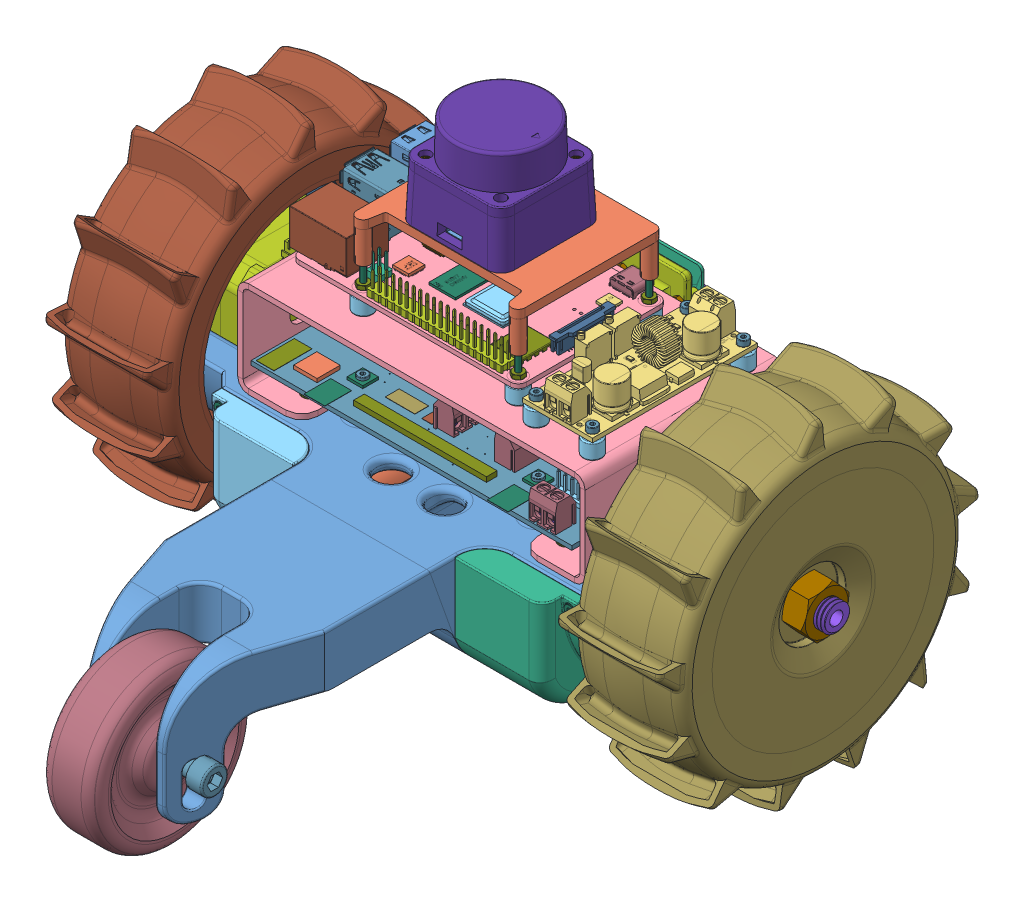
SolidWorks assembly RILey_assembly, configuration Default. Lengths in mm.
Overall size (244.39 192.08 262.82).
234 component instances, 82 part files, 220 mates.
Components (placement in the parent):
- MiddlepartV1-1: MiddlepartV1 [Middlepart_withoutTail] at origin size (201.11 74.9 106.82)
- MiddlepartV1-2: MiddlepartV1 [Tail] at origin size (60 50 93.64)
- 3_battery_pack-1: 3_battery_pack [Défaut] at (-114.6477 -13.5383 4.867) x (0.340955 0.94008 0) z (0.94008 -0.340955 0) size (33.05 64.4 54.62)
  - Li-ion Battery-1: Li-ion Battery [Défaut] at (13.1472 -31.5804 64) size (18 64.02 18)
  - link2-1: link2 [Défaut] at (30.5553 32.4196 84.2976) x (-0.340955 0 -0.94008) z (0 1 0) size (44 5 0.2)
  - Li-ion Battery-2: Li-ion Battery [Défaut] at (19.2844 -31.5804 80.9214) x (0.492149 0 0.870511) z (-0.870511 0 0.492149) size (18 64.02 18)
  - Li-ion Battery-3: Li-ion Battery [Défaut] at (25.4216 -31.5804 97.8429) x (0.922234 0 -0.386631) z (0.386631 0 0.922234) size (18 64.02 18)
  - link2-2: link2 [Défaut] at (25.7705 -31.5804 71.1051) x (0.340955 0 0.94008) z (0 -1 0) size (44 5 0.2)
- 3_battery_pack-2: 3_battery_pack [Défaut] at (-50.6477 -13.5383 4.867) x (0.340955 0.94008 0) z (0.94008 -0.340955 0) size (33.05 64.4 54.62)
  - Li-ion Battery-1: Li-ion Battery [Défaut] at (13.1472 -31.5804 64) size (18 64.02 18)
  - link2-1: link2 [Défaut] at (30.5553 32.4196 84.2976) x (-0.340955 0 -0.94008) z (0 1 0) size (44 5 0.2)
  - Li-ion Battery-2: Li-ion Battery [Défaut] at (19.2844 -31.5804 80.9214) x (0.492149 0 0.870511) z (-0.870511 0 0.492149) size (18 64.02 18)
  - Li-ion Battery-3: Li-ion Battery [Défaut] at (25.4216 -31.5804 97.8429) x (0.922234 0 -0.386631) z (0.386631 0 0.922234) size (18 64.02 18)
  - link2-2: link2 [Défaut] at (25.7705 -31.5804 71.1051) x (0.340955 0 0.94008) z (0 -1 0) size (44 5 0.2)
- BatteryCoverFront-1: BatteryCoverFront [Default] at (0 -39 -22) size (137.1 39.19 32.19)
- BatteryCoverBackLeft-1: BatteryCoverBackLeft [Default] at (-49.25 -40 30.5671) x (-1 0 0) z (0 0 -1) size (40.1 41.17 43.87)
- BatteryCoverBackRight-1: BatteryCoverBackRight [Default] at (49.25 -40 30.5671) x (-1 0 0) z (0 0 -1) size (40.1 41.17 43.86)
- Nema 17_Slim-1: Nema 17_Slim [Default] at (70.5 0 0) x (0 0 1) z (0 1 0) size (42 43 47.1)
- Nema 17_Slim-2: Nema 17_Slim [Default] at (-70.5 0 0) x (0 0 -1) z (0 1 0) size (42 43 47.1)
- LeftWheelAssembly-1: LeftWheelAssembly [Default] at (0.5 0 0) size (46.89 175.5 175.66)
  - HexBolt_modified-1: HexBolt_modified [Default] at (-101 0 0) x (0 0 1) z (-1 0 0) size (19.63 17 21.55)
  - hex nut style 1 gradeab_din-1: hex nut style 1 gradeab_din [Hexagon Nut ISO 4032 - M10 - D - S] at (-118.4 0 0) x (0 0 1) z (-1 0 0) size (16 18.48 8.4)
  - socket set screw cup point_din-1: socket set screw cup point_din [DIN 916 - M3 x 5-S] at (-104 7.5 0) x (0 -1 0) z (-0.467009 0 0.884252) size (5 3 3)
  - ReelyBuggyWheel_Left-2: ReelyBuggyWheel_Left [Default] at (-96.5 0 0) x (0 -0.851174 0.524883) z (-1 0 0) size (127.36 127.83 41.68)
- RightWheelAssembly-1: RightWheelAssembly [Default] at (68.7841 25.9686 -6.2213) x (-0.999996 0.002302 0.001897) z (-0.002983 -0.771739 -0.635933) size (47.18 164.08 164.48)
  - hex nut style 1 gradeab_din-2: hex nut style 1 gradeab_din [Hexagon Nut ISO 4032 - M10 - D - S] at (-40.7637 -21.3156 15.9632) x (0.002628 0.473226 -0.880937) z (0.999996 0 0.002983) size (16 18.48 8.4)
  - ReelyBuggyWheel_Right-1: ReelyBuggyWheel_Right [Default] at (-27.2638 -21.3156 16.0035) x (0.001045 0.936608 -0.350379) z (-0.999996 0 -0.002983) size (127.36 127.83 41.68)
  - socket set screw cup point_din-1: socket set screw cup point_din [DIN 916 - M3 x 5-S] at (-34.7467 -16.6097 10.2703) x (-0.002302 -0.635936 0.771739) z (-0.466048 0.683487 0.561824) size (5 3 3)
  - HexBolt_modified-1: HexBolt_modified [Default] at (-31.7638 -21.3156 15.9901) x (-0.001897 0.771742 0.635933) z (-0.999996 0 -0.002983) size (19.63 17 21.55)
- Backwheel-1: Backwheel [Default] at (0 -32.6496 136.5106) x (0 -0.126554 -0.99196) z (1 0 0) size (60 60 21)
- RILey_PCB-1: RILey_PCB [Default] at (48.6376 -44.5013 95.7539) x (-1 0 0) z (0 0 -1) size (120 19.05 71.04)
  - RILey_PCB.step-1: RILey_PCB.step [Default] at (-11.3624 54.5013 128.2539) x (1 0 0) z (0 1 0) size (120 71.04 11.3)
    - PCB Component.step-1: PCB Component.step [Default] at origin size (120 71.04 11.3)
      - Board.step-1: Board.step [Default] at origin size (120 70 1.57)
      - 0026604020.step-1: 0026604020.step [Default] at (95.25 66.04 1.57) size (7.77 10.01 0.1)
      - 0026604020.step-2: 0026604020.step [Default] at (26.67 66.04 1.57) size (7.77 10.01 0.1)
      - 2540-.step-1: 2540-.step [Default] at (61.27 63.5 1.57) size (49.68 3.96 1.83)
      - W237-102.step-1: W237-102.step [Default] at (11.481 64.491 1.57) x (-1 0 0) z (0 0 1) size (6.7 3.4 2.59)
      - W237-102.step-2: W237-102.step [Default] at (13.97 5.08 1.57) size (6.7 3.4 2.59)
      - W237-102.step-3: W237-102.step [Default] at (59.588 52.07 1.57) x (0 1 0) z (0 0 1) size (6.7 3.4 2.59)
      - W237-102.step-4: W237-102.step [Default] at (39.37 52.07 1.57) x (0 -1 0) z (0 0 1) size (6.7 3.4 2.59)
      - FE08-1_3D.step-1: FE08-1_3D.step [Default] at (26.67 31.75 1.57) x (0 1 0) z (0 0 1) size (20.82 2.5 11.3)
      - FE08-1_3D.step-2: FE08-1_3D.step [Default] at (12.7 31.75 1.57) x (0 1 0) z (0 0 1) size (20.82 2.5 11.3)
      - FE08-1_3D.step-3: FE08-1_3D.step [Default] at (93.98 27.94 1.57) x (0 -1 0) z (0 0 1) size (20.82 2.5 11.3)
      - FE08-1_3D.step-4: FE08-1_3D.step [Default] at (107.95 27.94 1.57) x (0 -1 0) z (0 0 1) size (20.82 2.5 11.3)
      - B4B-XH-A_LF__SN_.step-1: B4B-XH-A_LF__SN_.step [Default] at (5.08 27.94 1.57) x (0 1 0) z (0 0 1) size (12.9 6.25 0.1)
      - B4B-XH-A_LF__SN_.step-2: B4B-XH-A_LF__SN_.step [Default] at (115.57 31.75 1.57) x (0 -1 0) z (0 0 1) size (12.9 6.25 0.1)
      - 733980-62.step-1: 733980-62.step [Default] at (106.68 66.04 1.57) x (-1 0 0) z (0 0 1) size (8.75 8.65 1.36)
      - FE10-1_3D.step-1: FE10-1_3D.step [Default] at (66.04 15.259 1.57) x (0 -1 0) z (0 0 1) size (25.9 2.5 11.3)
      - FE04-1.step-1: FE04-1.step [Default] at (51.003 15.646 1.57) x (-1 0 0) z (0 0 1) size (10.16 2.5 11.3)
      - MA05-1_SMALLPAD.step-1: MA05-1_SMALLPAD.step [Default] at (13.97 55.88 1.57) x (-1 0 0) z (0 0 1) size (13.2 2.5 11)
      - 100uF.step-1: 100uF.step [Default] at (10.16 46.99 1.57) x (-1 0 0) z (0 0 1) size (7.55 7.55 0.1)
      - 100uF.step-2: 100uF.step [Default] at (97.79 43.18 1.57) size (7.55 7.55 0.1)
      - PTS18126V260.step-1: PTS18126V260.step [Default] at (62.23 40.64 0) x (0 1 0) z (0 0 -1) size (5.95 3.93 0.1)
      - MA04-1_SMALLPAD.step-1: MA04-1_SMALLPAD.step [Default] at (99.06 7.62 1.57) x (0 -1 0) z (0 0 1) size (10.66 2.5 11)
      - MA04-1_SMALLPAD.step-2: MA04-1_SMALLPAD.step [Default] at (104.14 7.62 1.57) x (0 -1 0) z (0 0 1) size (10.66 2.5 11)
      - MA04-1_SMALLPAD.step-3: MA04-1_SMALLPAD.step [Default] at (110.49 7.62 1.57) x (0 -1 0) z (0 0 1) size (10.66 2.5 11)
      - MA04-1_SMALLPAD.step-4: MA04-1_SMALLPAD.step [Default] at (115.57 7.62 1.57) x (0 -1 0) z (0 0 1) size (10.66 2.5 11)
      - MA04-1_SMALLPAD.step-5: MA04-1_SMALLPAD.step [Default] at (42.012 6.401 1.57) x (-1 0 0) z (0 0 1) size (10.66 2.5 11)
      - 1uF.step-1: 1uF.step [Default] at (85.09 36.83 1.57) x (0 -1 0) z (0 0 1) size (4.14 1.6 1.07)
      - 47uF.step-1: 47uF.step [Default] at (80.01 38.1 1.57) x (0 -1 0) z (0 0 1) size (6.68 1.6 0.99)
      - SA5.0A-E3_54.step-1: SA5.0A-E3_54.step [Default] at (67.31 55.88 1.57) x (0 -1 0) z (0 0 1) size (21.18 3.8 0.1)
      - IRF9530NPBF.step-1: IRF9530NPBF.step [Default] at (74.93 53.34 1.57) size (11.04 5.19 0.1)
      - BCM857BS,115.step-1: BCM857BS,115.step [Default] at (78.74 48.26 0) x (1 0 0) z (0 0 -1) size (3.4 2.7 0.1)
      - 10k.step-1: 10k.step [Default] at (74.93 40.64 1.57) x (0 1 0) z (0 0 1) size (10.6 2.5 4.42)
      - 10k.step-2: 10k.step [Default] at (72.39 40.64 1.57) x (0 1 0) z (0 0 1) size (10.6 2.5 4.42)
      - 2,8.step-1: 2,8.step [Default] at (27.15 9.65 1.57) size (5.84 5.84 0.97)
      - 2,8.step-2: 2,8.step [Default] at (92.85 55.35 1.57) size (5.84 5.84 0.97)
      - 2,8.step-3: 2,8.step [Default] at (27.15 55.35 1.57) size (5.84 5.84 0.97)
      - 2,8.step-4: 2,8.step [Default] at (92.85 9.65 1.57) size (5.84 5.84 0.97)
      - 1101M2S3CQE2.step-1: 1101M2S3CQE2.step [Default] at (115.621 62.763 1.57) size (6.6 14.23 0.1)
  - DRV 8825 With Headers Assem-1: DRV 8825 With Headers Assem [Default] at (18.6208 50.4495 104.6201) x (0 0 -1) z (0 1 0) size (21 15 10.9)
    - PCB-1: PCB [Default] at (8.1162 10.2982 16.4218) size (21 15 1.8)
    - SMD Pot-1: SMD Pot [Default] at (-0.2134 7.4613 18.0218) x (0 -1 0) z (0 0 1) size (3 3 1.3)
    - 0603 Resistor-1: 0603 Resistor [Default] at (-1.0068 10.8561 18.0218) size (1.5 0.8 0.5)
    - 0603 Resistor-2: 0603 Resistor [Default] at (-1.0286 12.2306 18.0218) size (1.5 0.8 0.5)
    - 0805 Capacitor-1: 0805 Capacitor [Default] at (-0.8941 14.0417 18.0218) size (2 1.25 1.25)
    - 0402 Resistor-1: 0402 Resistor [Default] at (16.8896 6.6863 18.0218) x (0 -1 0) z (0 0 1) size (1 0.68 0.66)
    - 0402 Resistor-2: 0402 Resistor [Default] at (16.8896 10.308 18.0218) x (0 -1 0) z (0 0 1) size (1 0.68 0.66)
    - 0402 Resistor-3: 0402 Resistor [Default] at (16.8896 13.6408 18.0218) x (0 -1 0) z (0 0 1) size (1 0.68 0.66)
    - 0402 Resistor-4: 0402 Resistor [Default] at (6.8882 6.5987 18.0218) x (0 -1 0) z (0 0 1) size (1 0.68 0.66)
    - 0402 Resistor-5: 0402 Resistor [Default] at (5.9719 6.5987 18.0218) x (0 -1 0) z (0 0 1) size (1 0.68 0.66)
    - 0402 Resistor-6: 0402 Resistor [Default] at (5.456 14.3274 18.0218) size (1 0.68 0.66)
    - 0402 Resistor-7: 0402 Resistor [Default] at (5.456 13.4855 18.0218) size (1 0.68 0.66)
    - DRV8825 IC-1: DRV8825 IC [Default] at (11.7347 10.2312 18.0218) x (0 -1 0) z (0 0 1) size (9.6 6.2 1.2)
    - 8 pin Header-1: 8 pin Header [Default] at (8.1162 16.2982 13.9218) size (21 2.5 10.5)
    - 8 pin Header-2: 8 pin Header [Default] at (8.1162 4.2982 13.9218) size (21 2.5 10.5)
  - DRV 8825 With Headers Assem-2: DRV 8825 With Headers Assem [Default] at (79.3044 50.4495 92.1976) x (0 0 1) z (0 1 0) size (21 15 10.9)
    - PCB-1: PCB [Default] at (8.1162 10.2982 16.4218) size (21 15 1.8)
    - SMD Pot-1: SMD Pot [Default] at (-0.2134 7.4613 18.0218) x (0 -1 0) z (0 0 1) size (3 3 1.3)
    - 0603 Resistor-1: 0603 Resistor [Default] at (-1.0068 10.8561 18.0218) size (1.5 0.8 0.5)
    - 0603 Resistor-2: 0603 Resistor [Default] at (-1.0286 12.2306 18.0218) size (1.5 0.8 0.5)
    - 0805 Capacitor-1: 0805 Capacitor [Default] at (-0.8941 14.0417 18.0218) size (2 1.25 1.25)
    - 0402 Resistor-1: 0402 Resistor [Default] at (16.8896 6.6863 18.0218) x (0 -1 0) z (0 0 1) size (1 0.68 0.66)
    - 0402 Resistor-2: 0402 Resistor [Default] at (16.8896 10.308 18.0218) x (0 -1 0) z (0 0 1) size (1 0.68 0.66)
    - 0402 Resistor-3: 0402 Resistor [Default] at (16.8896 13.6408 18.0218) x (0 -1 0) z (0 0 1) size (1 0.68 0.66)
    - 0402 Resistor-4: 0402 Resistor [Default] at (6.8882 6.5987 18.0218) x (0 -1 0) z (0 0 1) size (1 0.68 0.66)
    - 0402 Resistor-5: 0402 Resistor [Default] at (5.9719 6.5987 18.0218) x (0 -1 0) z (0 0 1) size (1 0.68 0.66)
    - 0402 Resistor-6: 0402 Resistor [Default] at (5.456 14.3274 18.0218) size (1 0.68 0.66)
    - 0402 Resistor-7: 0402 Resistor [Default] at (5.456 13.4855 18.0218) size (1 0.68 0.66)
    - DRV8825 IC-1: DRV8825 IC [Default] at (11.7347 10.2312 18.0218) x (0 -1 0) z (0 0 1) size (9.6 6.2 1.2)
    - 8 pin Header-1: 8 pin Header [Default] at (8.1162 16.2982 13.9218) size (21 2.5 10.5)
    - 8 pin Header-2: 8 pin Header [Default] at (8.1162 4.2982 13.9218) size (21 2.5 10.5)
  - MPU9250.STEP-2: MPU9250.STEP [Default] at (87.1776 67.9346 116.1747) x (0 0 1) z (-1 0 0) size (26 3.91 16)
    - PCB.STEP-1: PCB.STEP [Default] at (-2.9998 1.0768 26) size (26 2.2 16)
    - C2.STEP-1: C2.STEP [Default] at (-2.4989 2.0768 21) x (0 0 -1) z (1 0 0) size (2 1.81 5.01)
    - MP92.STEP-1: MP92.STEP [Default] at (-2.9998 1.0968 25.5) x (0 0 -1) z (1 0 0) size (3.29 1.01 3.29)
    - C1_Predeterminado_Como mecanizada_.STEP-1: C1_Predeterminado_Como mecanizada_.STEP [Default] at (2.1384 1.0968 23.0905) x (0 0 1) z (-1 0 0) size (2.2 0.83 0.9)
    - C1_Predeterminado_Como mecanizada_.STEP-2: C1_Predeterminado_Como mecanizada_.STEP [Default] at (0.9102 1.0968 27.1044) x (0 0 1) z (-1 0 0) size (2.2 0.83 0.9)
    - C1_Predeterminado_Como mecanizada_.STEP-3: C1_Predeterminado_Como mecanizada_.STEP [Default] at (0.9102 1.0968 23.0905) x (0 0 1) z (-1 0 0) size (2.2 0.83 0.9)
    - C1_Predeterminado_Como mecanizada_.STEP-4: C1_Predeterminado_Como mecanizada_.STEP [Default] at (-8.3098 1.0968 23.0905) x (0 0 1) z (-1 0 0) size (2.2 0.83 0.9)
    - C1_Predeterminado_Como mecanizada_.STEP-5: C1_Predeterminado_Como mecanizada_.STEP [Default] at (-9.7098 1.0968 27.1044) x (0 0 1) z (-1 0 0) size (2.2 0.83 0.9)
    - R1.STEP-1: R1.STEP [Default] at (3.5484 1.1168 27.2144) x (0 0 -1) z (1 0 0) size (2.2 0.47 0.9)
    - R1.STEP-2: R1.STEP [Default] at (2.1484 1.1168 27.2144) x (0 0 -1) z (1 0 0) size (2.2 0.47 0.9)
    - R1.STEP-3: R1.STEP [Default] at (-6.8998 1.1168 23.2005) x (0 0 -1) z (1 0 0) size (2.2 0.47 0.9)
    - R1.STEP-4: R1.STEP [Default] at (-8.2998 1.1168 27.2144) x (0 0 -1) z (1 0 0) size (2.2 0.47 0.9)
    - R1.STEP-5: R1.STEP [Default] at (-6.8998 1.1168 27.2144) x (0 0 -1) z (1 0 0) size (2.2 0.47 0.9)
    - V1.STEP-1: V1.STEP [Default] at (-13.0785 1.5868 25.9) size (2.9 0.96 3.2)
  - PinHeader10row-1: PinHeader10row [Default] at (53.4076 66.9113 102.8349) x (0 0 -1) z (-1 0 0) size (25.4 11.54 2.54)
  - DG301-5.0-02-1: DG301-5.0-02 [Default] at (0.1076 56.0713 125.1439) x (1 0 0) z (0 1 0) size (10.6 7.6 14.3)
  - DG301-5.0-02-2: DG301-5.0-02 [Default] at (27.4376 56.0713 78.6839) x (0 0 -1) z (0 1 0) size (10.6 7.6 14.3)
  - DG301-5.0-02-3: DG301-5.0-02 [Default] at (48.7956 56.0713 73.6839) x (0 0 1) z (0 1 0) size (10.6 7.6 14.3)
  - DG301-5.0-02-4: DG301-5.0-02 [Default] at (2.6186 56.0713 61.7929) x (-1 0 0) z (0 1 0) size (10.6 7.6 14.3)
- 3rdFloorAssembly-1: 3rdFloorAssembly [Default] at origin size (130 100.19 75)
  - socket head cap screw 4762_din-1: socket head cap screw 4762_din [EN ISO 4762 M2 x 12 - 12S] at (37.5 45.65 -28.25) x (0 -1 0) z (0 0 1) size (14 3.8 3.8)
  - socket head cap screw 4762_din-2: socket head cap screw 4762_din [EN ISO 4762 M2 x 12 - 12S] at (58.5 45.65 -28.25) x (0 -1 0) z (0 0 1) size (14 3.8 3.8)
  - socket head cap screw 4762_din-3: socket head cap screw 4762_din [EN ISO 4762 M2 x 12 - 12S] at (58.5 45.65 28.25) x (0 -1 0) z (0 0 1) size (14 3.8 3.8)
  - socket head cap screw 4762_din-4: socket head cap screw 4762_din [EN ISO 4762 M2 x 12 - 12S] at (37.5 45.65 28.25) x (0 -1 0) z (0 0 1) size (14 3.8 3.8)
  - socket head cap screw_iso-1: socket head cap screw_iso [ISO 4762 M2 x 20 - 20C] at (-31 32 -24.5) x (0 1 0) z (0 0 1) size (22 3.8 3.8)
  - socket head cap screw_iso-2: socket head cap screw_iso [ISO 4762 M2 x 20 - 20C] at (-31 32 24.5) x (0 1 0) z (0 0 1) size (22 3.8 3.8)
  - socket head cap screw_iso-3: socket head cap screw_iso [ISO 4762 M2 x 20 - 20C] at (27 32 -24.5) x (0 1 0) z (0 0 1) size (22 3.8 3.8)
  - socket head cap screw_iso-4: socket head cap screw_iso [ISO 4762 M2 x 20 - 20C] at (27 32 24.5) x (0 1 0) z (0 0 1) size (22 3.8 3.8)
  - hex nut style 1 gradeab_iso-1: hex nut style 1 gradeab_iso [ISO - 4032 - M2 - W - C] at (-31 45.19 -24.5) x (1 0 0) z (0 1 0) size (4 4.62 1.6)
  - hex nut style 1 gradeab_iso-2: hex nut style 1 gradeab_iso [ISO - 4032 - M2 - W - C] at (27 45.19 -24.5) x (1 0 0) z (0 1 0) size (4 4.62 1.6)
  - hex nut style 1 gradeab_iso-3: hex nut style 1 gradeab_iso [ISO - 4032 - M2 - W - C] at (-31 45.19 24.5) x (1 0 0) z (0 1 0) size (4 4.62 1.6)
  - hex nut style 1 gradeab_iso-4: hex nut style 1 gradeab_iso [ISO - 4032 - M2 - W - C] at (27 45.19 24.5) x (1 0 0) z (0 1 0) size (4 4.62 1.6)
  - hex nut style 1 gradeab_iso-5: hex nut style 1 gradeab_iso [ISO - 4032 - M2 - W - C] at (58.5 32.4 -28.25) x (1 0 0) z (0 -1 0) size (4 4.62 1.6)
  - hex nut style 1 gradeab_iso-6: hex nut style 1 gradeab_iso [ISO - 4032 - M2 - W - C] at (37.5 32.4 -28.25) x (1 0 0) z (0 -1 0) size (4 4.62 1.6)
  - hex nut style 1 gradeab_iso-7: hex nut style 1 gradeab_iso [ISO - 4032 - M2 - W - C] at (37.5 32.4 28.25) x (1 0 0) z (0 -1 0) size (4 4.62 1.6)
  - hex nut style 1 gradeab_iso-8: hex nut style 1 gradeab_iso [ISO - 4032 - M2 - W - C] at (58.5 32.4 28.25) x (1 0 0) z (0 -1 0) size (4 4.62 1.6)
  - LD06_Assembly-1: LD06_Assembly [Default] at (-60.828 42.1202 31.9351) x (0 0 -1) z (1 0 0) size (54 48.5 63)
    - LD06_LiDAR-1: LD06_LiDAR [Default] at (15.6414 21.3154 28.1688) size (38.59 33.3 38.59)
      - LD06_LiDAR-1: LD06_LiDAR [Default] at (16.3187 3.4544 28.6342) size (38.59 33.3 38.59)
      - JIS_B1111_M2x6.step-1: JIS_B1111_M2x6.step [Default] at (30.4187 21.1806 42.7342) x (1 0 0) z (0 1 0) size (3.5 3.5 7.3)
      - JIS_B1111_M2x6.step-2: JIS_B1111_M2x6.step [Default] at (2.2187 21.1806 14.5342) x (1 0 0) z (0 1 0) size (3.5 3.5 7.3)
      - jst-1.5mm-4P.step-1: jst-1.5mm-4P.step [Default] at (4.0237 7.1794 28.6342) x (0 0 -1) z (0 1 0) size (7.5 7.2 3.5)
    - LD06_PiBracket-1: LD06_PiBracket [Default] at (31.9351 21.5698 58.828) x (0 0 1) z (-1 0 0) size (63 27 54)
  - dc-dc-5a-cc-merged-1: dc-dc-5a-cc-merged [Default] at (48 43.6 0) x (0 0 -1) z (1 0 0) size (61.7 17.87 26.2)
  - Raspberry Pi 4 Model B-1: Raspberry Pi 4 Model B [Default] at (-12 42.8 0) x (-1 0 0) z (0 0 -1) size (88.99 19.9 58.4)
    - PCB, RPi4ModelB-1: PCB, RPi4ModelB [Default] at origin size (85 1.6 56)
    - Broadcom BCM2711B0 CPU, RPi4ModelB-1: Broadcom BCM2711B0 CPU, RPi4ModelB [Default] at (-13.25 0.8 -4.5) size (15 2.3 15)
    - 2.54 mm DUPONT MALE PIN HEADER, POE, 2X2, RPi4ModelB-1: 2.54 mm DUPONT MALE PIN HEADER, POE, 2X2, RPi4ModelB [Default] at (19 0.8 -18.5) size (5.08 11.3 5.08)
    - 2.54 mm DUPONT MALE PIN HEADER, IO, 2X20, RPi4ModelB-1: 2.54 mm DUPONT MALE PIN HEADER, IO, 2X20, RPi4ModelB [Default] at (-10 0.8 -24.5) size (50.8 11.3 5.08)
    - Camera Connector, RPi4ModelB-1: Camera Connector, RPi4ModelB [Default] at (4 0.8 16.5) x (0 0 -1) z (1 0 0) size (22.4 5.68 5.07)
    - Microphone Plug, RPi4ModelB-1: Microphone Plug, RPi4ModelB [Default] at (11.5 0.8 21.65) size (7.23 7.55 15)
    - Display Connector, RPi4ModelB-1: Display Connector, RPi4ModelB [Default] at (-38.5 0.8 0) x (0 0 1) z (-1 0 0) size (22.4 5.68 5.07)
    - Gigabit Ethernet Port, RPi4ModelB-1: Gigabit Ethernet Port, RPi4ModelB [Default] at (45.5 7.55 -17.75) x (0 0 -1) z (1 0 0) size (16.2 17.24 21.64)
    - Female Micro HDMI Connector, RPi4ModelB-2: Female Micro HDMI Connector, RPi4ModelB [Default] at (-3 0.8 27.3875) size (6.5 3.51 7.5)
    - Female Micro HDMI Connector, RPi4ModelB-3: Female Micro HDMI Connector, RPi4ModelB [Default] at (-16.5 0.8 27.3875) size (6.5 3.51 7.5)
    - Female USB Type C Connector, RPi4ModelB-1: Female USB Type C Connector, RPi4ModelB [Default] at (-31.3 0.8 26.5419) size (8.94 3.96 7.9)
    - 2X USB3.0 PORTS, RPi4ModelB-2: 2X USB3.0 PORTS, RPi4ModelB [Default] at (37.07 0.8 1) size (17.47 19.41 15.68)
    - 91D77 D9WHV 778K, 4 GB LPDDR4 SDRAM, RPi4ModelB-1: 91D77 D9WHV 778K, 4 GB LPDDR4 SDRAM, RPi4ModelB [Default] at (2.25 0.8 -4.5) size (10 0.8 14.5)
    - Cypress CYW43455 Wireless Module Cover, RPi4ModelB-1: Cypress CYW43455 Wireless Module Cover, RPi4ModelB [Default] at (-30.5 0.8 -14.5) size (11 1.6 13)
    - SD Card Slot, RPi4ModelB-1: SD Card Slot, RPi4ModelB [Default] at (-35.3 -0.8 0) x (0 0 -1) z (-1 0 0) size (11.95 1.45 11.4)
    - VIA VL805 PCIe USB 3.0 controller, RPi4ModelB-1: VIA VL805 PCIe USB 3.0 controller, RPi4ModelB [Default] at (17.5 0.8 4) size (8.8 0.8 8.8)
    - 2X USB2.0 PORTS, RPi4ModelB-1: 2X USB2.0 PORTS, RPi4ModelB [Default] at (37.065 0.65 19) size (17.87 19.16 15.33)
    - Broadcom BCM54213PE Gigabit Ethernet Transceiver, RPi4ModelB-1: Broadcom BCM54213PE Gigabit Ethernet Transceiver, RPi4ModelB [Default] at (16.5 0.8 -10) size (6.8 1 6.8)
    - MxL7704 Universal PMIC, RPi4ModelB-1: MxL7704 Universal PMIC, RPi4ModelB [Default] at (-32.5 0.8 16) size (5.4 0.8 5.4)
  - 3rdFloor_Sheetmetal-1: 3rdFloor_Sheetmetal [Default] at (0 36 0) size (130 36 75)
  - Spacer-1: Spacer [Default] at (37.5 36 -28.25) x (-0.470741 0 0.882271) z (-0.882271 0 -0.470741) size (7 6 7)
  - Spacer-2: Spacer [Default] at (58.5 36 -28.25) x (0.784801 0 0.619748) z (-0.619748 0 0.784801) size (7 6 7)
  - Spacer-3: Spacer [Default] at (-31 36 24.5) size (7 6 7)
  - Spacer-4: Spacer [Default] at (37.5 36 28.25) x (0.517299 0 -0.855805) z (0.855805 0 0.517299) size (7 6 7)
  - Spacer-5: Spacer [Default] at (58.5 36 28.25) size (7 6 7)
  - Spacer-6: Spacer [Default] at (27 36.3 -24.5) x (-0.705828 0 0.708384) z (-0.708384 0 -0.705828) size (7 6 7)
  - Spacer-7: Spacer [Default] at (27 36 24.5) x (0.999844 0 -0.017672) z (0.017672 0 0.999844) size (7 6 7)
  - Spacer-8: Spacer [Default] at (-31 36 -24.5) x (-0.657111 0 -0.753794) z (0.753794 0 -0.657111) size (7 6 7)
- CameraAssembly-1: CameraAssembly [Default] at (0 -2.8393 -0.3795) x (1 0 0) z (0 -0.077018 0.99703) size (25.31 32.26 33.3)
  - Cam V2.1 v1.step-1: Cam V2.1 v1.step [Default] at (0 16.3492 -59.3807) x (0 -0.098914 -0.995096) z (-1 0 0) size (6.45 24 25)
  - CameraMount-1: CameraMount [Default] at (-12.5 4.7048 -55.2085) x (1 0 0) z (0 0.098914 0.995096) size (25.31 30.03 24.03)
  - socket head cap screw_din-1: socket head cap screw_din [DIN 912 M2 x 10 --- 10S] at (-10.5 18.5402 -62.6133) x (0 0.098914 0.995096) z (-0.995096 -0.098429 0.009784) size (12 3.8 3.8)
  - socket head cap screw_din-2: socket head cap screw_din [DIN 912 M2 x 10 --- 10S] at (-10.5 6.1015 -61.3769) x (0 0.098914 0.995096) z (-0.995096 -0.098429 0.009784) size (12 3.8 3.8)
  - socket head cap screw_din-3: socket head cap screw_din [DIN 912 M2 x 10 --- 10S] at (10.5 6.1015 -61.3769) x (0 0.098914 0.995096) z (-0.995096 -0.098429 0.009784) size (12 3.8 3.8)
  - socket head cap screw_din-4: socket head cap screw_din [DIN 912 M2 x 10 --- 10S] at (10.5 18.5402 -62.6133) x (0 0.098914 0.995096) z (-0.995096 -0.098429 0.009784) size (12 3.8 3.8)
  - hex nut style 1 gradeab_din-1: hex nut style 1 gradeab_din [Hexagon Nut ISO 4032 - M2 - D - S] at (-10.5 19.5887 -52.0653) x (1 0 0) z (0 0.098914 0.995096) size (4 4.62 1.6)
  - hex nut style 1 gradeab_din-2: hex nut style 1 gradeab_din [Hexagon Nut ISO 4032 - M2 - D - S] at (10.5 19.5887 -52.0653) x (1 0 0) z (0 0.098914 0.995096) size (4 4.62 1.6)
  - hex nut style 1 gradeab_din-3: hex nut style 1 gradeab_din [Hexagon Nut ISO 4032 - M2 - D - S] at (-10.5 7.15 -50.8289) x (1 0 0) z (0 0.098914 0.995096) size (4 4.62 1.6)
  - hex nut style 1 gradeab_din-4: hex nut style 1 gradeab_din [Hexagon Nut ISO 4032 - M2 - D - S] at (10.5 7.15 -50.8289) x (1 0 0) z (0 0.098914 0.995096) size (4 4.62 1.6)
  - Cam V2.1 v1.step-2: Cam V2.1 v1.step [Default] at (0 16.3492 -59.3807) x (0 -0.098914 -0.995096) z (-1 0 0) size (6.45 24 25)
- TimeOfFlightAssembly-1: TimeOfFlightAssembly [Default] at (0 38.8219 -25.9653) x (-1 0 0) z (0 0.924225 0.381849) size (28 16.66 17.76)
  - TimeOfFlightMount-1: TimeOfFlightMount [Default] at (0 -3.6203 -48.3357) x (-1 0 0) z (0 -0.87922 0.476417) size (28 12 8.25)
  - VL53l1X-1: VL53l1X [Varsayılan] at (0 -6.8924 -51.2259) x (-1 0 0) z (0 -0.87922 0.476417) size (25 4 10.5)
  - hex nut style 1 gradeab_iso-1: hex nut style 1 gradeab_iso [ISO - 4032 - M3 - W - N] at (-10 -3.7957 -45.511) x (1 0 0) z (0 0.476417 0.87922) size (5.5 6.35 2.4)
  - hex nut style 1 gradeab_iso-2: hex nut style 1 gradeab_iso [ISO - 4032 - M3 - W - N] at (10 -3.7957 -45.511) x (-0.997793 -0.058376 0.031632) z (0 0.476417 0.87922) size (5.5 6.35 2.4)
  - socket head cap screw_iso-1: socket head cap screw_iso [ISO 4762 M3 x 8 - 8C] at (-10 -9.0839 -55.2703) x (0 0.476417 0.87922) z (-0.87922 -0.418875 0.226973) size (11 5.5 5.5)
  - socket head cap screw_iso-2: socket head cap screw_iso [ISO 4762 M3 x 8 - 8C] at (10 -9.0839 -55.2703) x (0 0.476417 0.87922) z (-0.87922 -0.418875 0.226973) size (11 5.5 5.5)
- socket head cap screw 4762_din-2: socket head cap screw 4762_din [EN ISO 4762 M3 x 8 - 8C] at (-103.5 -15.5 -15.5) x (1 0 0) z (0 -0.158197 0.987408) size (11 5.5 5.5)
- socket head cap screw 4762_din-3: socket head cap screw 4762_din [EN ISO 4762 M3 x 8 - 8C] at (-103.5 15.5 -15.5) size (11 5.5 5.5)
- socket head cap screw 4762_din-4: socket head cap screw 4762_din [EN ISO 4762 M3 x 8 - 8C] at (-103.5 15.5 15.5) size (11 5.5 5.5)
- socket head cap screw 4762_din-5: socket head cap screw 4762_din [EN ISO 4762 M3 x 8 - 8C] at (-103.5 -15.5 15.5) size (11 5.5 5.5)
- socket head cap screw 4762_din-6: socket head cap screw 4762_din [EN ISO 4762 M3 x 8 - 8C] at (103.5 15.5 -15.5) x (-1 0 0) z (0 0.924225 0.381849) size (11 5.5 5.5)
- socket head cap screw 4762_din-7: socket head cap screw 4762_din [EN ISO 4762 M3 x 8 - 8C] at (103.5 -15.5 -15.5) x (-1 0 0) z (0 0.924225 0.381849) size (11 5.5 5.5)
- socket head cap screw 4762_din-8: socket head cap screw 4762_din [EN ISO 4762 M3 x 8 - 8C] at (103.5 -15.5 15.5) x (-1 0 0) z (0 0.924225 0.381849) size (11 5.5 5.5)
- socket head cap screw 4762_din-9: socket head cap screw 4762_din [EN ISO 4762 M3 x 8 - 8C] at (103.5 15.5 15.5) x (-1 0 0) z (0 0.924225 0.381849) size (11 5.5 5.5)
- socket head cap screw 4762_din-16: socket head cap screw 4762_din [EN ISO 4762 M2 x 6 - 6C] at (93.7423 0 0) size (8 3.8 3.8)
- socket head cap screw 4762_din-22: socket head cap screw 4762_din [EN ISO 4762 M2 x 6 - 6C] at (-32.85 13.57 -22.85) x (0 -1 0) z (0 0 1) size (8 3.8 3.8)
- socket head cap screw 4762_din-25: socket head cap screw 4762_din [EN ISO 4762 M2 x 6 - 6C] at (32.85 13.57 -22.85) x (0 -1 0) z (0 0 1) size (8 3.8 3.8)
- socket head cap screw 4762_din-26: socket head cap screw 4762_din [EN ISO 4762 M2 x 6 - 6C] at (32.85 13.57 22.85) x (0 -1 0) z (0 0 1) size (8 3.8 3.8)
- socket head cap screw 4762_din-27: socket head cap screw 4762_din [EN ISO 4762 M2 x 6 - 6C] at (-32.85 13.57 22.85) x (0 -1 0) z (0 0 1) size (8 3.8 3.8)
- socket head cap screw 4762_din-32: socket head cap screw 4762_din [EN ISO 4762 M2 x 12 - 12C] at (7 3.5 -37) x (-1 0 0) z (0 0.793454 0.60863) size (14 3.8 3.8)
- socket head cap screw 4762_din-33: socket head cap screw 4762_din [EN ISO 4762 M2 x 12 - 12C] at (-7 -1 -43.5) size (14 3.8 3.8)
- socket head cap screw 4762_din-58: socket head cap screw 4762_din [EN ISO 4762 M3 x 10 - 10S] at (48 -8 -27.5) x (0 1 0) z (0 0 1) size (13 5.5 5.5)
- socket head cap screw 4762_din-59: socket head cap screw 4762_din [EN ISO 4762 M3 x 10 - 10S] at (-48 -8 -27.5) x (0 1 0) z (0 0 1) size (13 5.5 5.5)
- socket head cap screw 4762_din-61: socket head cap screw 4762_din [EN ISO 4762 M3 x 10 - 10S] at (-48 -8 27.5) x (0 1 0) z (0 0 1) size (13 5.5 5.5)
- socket head cap screw 4762_din-62: socket head cap screw 4762_din [EN ISO 4762 M3 x 10 - 10S] at (48 -8 27.5) x (0 1 0) z (0 0 1) size (13 5.5 5.5)
- socket head cap screw 4762_din-66: socket head cap screw 4762_din [EN ISO 4762 M6 x 45 - 24S] at (25.4965 -32.6496 136.5106) x (-1 0 0) z (0 0.999134 -0.041605) size (51 10 10)
- socket head cap screw_iso-9: socket head cap screw_iso [ISO 4762 M2 x 10 - 10C] at (65.5 -3.5 -44) x (0 0 1) z (-0.626245 0.779626 0) size (12 3.8 3.8)
- socket head cap screw_iso-13: socket head cap screw_iso [ISO 4762 M2 x 10 - 10C] at (-65.5 -3.5 -44) x (0 0 1) z (0.96474 -0.263204 0) size (12 3.8 3.8)
- socket head cap screw_iso-15: socket head cap screw_iso [ISO 4762 M2 x 16 - 16C] at (-65.5 -36.5 -24) x (0 0 1) z (0.512332 0.858787 0) size (18 3.8 3.8)
- socket head cap screw_iso-16: socket head cap screw_iso [ISO 4762 M2 x 16 - 16C] at (65.5 -36.5 -24) x (0 0 1) z (-0.779626 -0.626245 0) size (18 3.8 3.8)
- socket head cap screw_iso-17: socket head cap screw_iso [ISO 4762 M2 x 16 - 16C] at (0 -36.5 -24) x (0 0 1) z (-0.932157 0.362053 0) size (18 3.8 3.8)
- socket head cap screw_iso-19: socket head cap screw_iso [ISO 4762 M2 x 16 - 16C] at (65.5 -36.5 25.0671) x (0 0 -1) z (1 0 0) size (18 3.8 3.8)
- socket head cap screw_iso-20: socket head cap screw_iso [ISO 4762 M2 x 16 - 16C] at (-65.5 -36.5 25.0671) x (0 0 -1) z (1 0 0) size (18 3.8 3.8)
- socket head cap screw_iso-22: socket head cap screw_iso [ISO 4762 M2 x 10 - 10C] at (65.5 -3.5 44.0671) x (0 0 -1) z (1 0 0) size (12 3.8 3.8)
- socket head cap screw_iso-23: socket head cap screw_iso [ISO 4762 M2 x 10 - 10C] at (-65.5 -3.5 44.0671) x (0 0 -1) z (1 0 0) size (12 3.8 3.8)
- socket head cap screw_iso-26: socket head cap screw_iso [ISO 4762 M5 x 30 - 22C] at (-19 -15 44) x (0 0 1) z (-1 0 0) size (35 8.5 8.5)
- socket head cap screw_iso-27: socket head cap screw_iso [ISO 4762 M5 x 30 - 22C] at (19 -15 44) x (0 0 1) z (-1 0 0) size (35 8.5 8.5)
- hex nut style 1 gradeab_iso-11: hex nut style 1 gradeab_iso [ISO - 4032 - M2 - W - C] at (6.6 -0.8982 -43.5681) x (0 0.568605 0.822611) z (1 0 0) size (4 4.62 1.6)
- hex nut style 1 gradeab_iso-16: hex nut style 1 gradeab_iso [ISO - 4032 - M2 - W - C] at (-6.6 3.5 -37) x (0 0.591276 0.80647) z (-1 0 0) size (4 4.62 1.6)
- hex nut style 1 gradeab_iso-21: hex nut style 1 gradeab_iso [ISO - 4032 - M3 - W - C] at (48 4.4 27.5) x (1 0 0) z (0 1 0) size (5.5 6.35 2.4)
- hex nut style 1 gradeab_iso-22: hex nut style 1 gradeab_iso [ISO - 4032 - M3 - W - C] at (-48 4.4 27.5) x (1 0 0) z (0 1 0) size (5.5 6.35 2.4)
- hex nut style 1 gradeab_iso-23: hex nut style 1 gradeab_iso [ISO - 4032 - M3 - W - C] at (-48 4.4 -27.5) x (1 0 0) z (0 1 0) size (5.5 6.35 2.4)
- hex nut style 1 gradeab_iso-24: hex nut style 1 gradeab_iso [ISO - 4032 - M3 - W - C] at (48 4.4 -27.5) x (1 0 0) z (0 1 0) size (5.5 6.35 2.4)
- hex nut style 1 gradeab_iso-26: hex nut style 1 gradeab_iso [ISO - 4032 - M6 - W - C] at (-24.6965 -32.6496 136.5106) x (0 -0.97715 0.212551) z (-1 0 0) size (10 11.55 5.2)
Mates (geometry in assembly coordinates):
- Concentric3: concentric anti-aligned: cylinder of MiddlepartV1-1 through (-84.1863 0 0) axis (-1 0 0) radius 4; cylinder of Step NEMA 17-2/aVratilo-1 through (-96.5 0 0) axis (1 0 0) radius 2.5
- Concentric4: concentric anti-aligned: cylinder of MiddlepartV1-1 through (-106.8137 0 0) axis (1 0 0) radius 4; cylinder of Step NEMA 17-1/aVratilo-1 through (96.5 0 0) axis (-1 0 0) radius 2.5
- Concentric5: concentric aligned: cylinder of MiddlepartV1-1 through (89.8431 15.5 15.5) axis (1 0 0) radius 2; circle of Step NEMA 17-1/aGornji dr_a -1
- Coincident5: coincident anti-aligned: plane of MiddlepartV1-1 through (-61.5 -32 45) normal (0 1 0); plane of Battery_mockup-1 through (0 -32 -12.4155) normal (0 -1 0)
- Width1: width aligned: plane of MiddlepartV1-1 through (-61.5 -5 45) normal (1 0 0); plane of MiddlepartV1-1 through (61.5 -5 45) normal (-1 0 0); plane of Battery_mockup-1 through (28 -7 -47.4155) normal (1 0 0); plane of Battery_mockup-1 through (-28 -7 -47.4155) normal (-1 0 0)
- Coincident6: coincident anti-aligned: plane of MiddlepartV1-1 through (-95.5 40 -40) normal (1 0 0); plane of Step NEMA 17-2/aGornji dr_a -1 through (-72.5 0 0) normal (-1 0 0)
- Coincident7: coincident anti-aligned: plane of MiddlepartV1-1 through (95.5 40 -40) normal (-1 0 0); plane of Step NEMA 17-1/aGornji dr_a -1 through (72.5 0 0) normal (1 0 0)
- Concentric6: concentric anti-aligned: cylinder of Step NEMA 17-2/aVratilo-1 through (-96.5 0 0) axis (1 0 0) radius 2.5; cylinder of wiel-2 through (-111.5665 0 0) axis (-1 0 0) radius 9.5
- Concentric7: concentric anti-aligned: cylinder of Step NEMA 17-1/aVratilo-1 through (96.5 0 0) axis (-1 0 0) radius 2.5; cylinder of wiel-1 through (104.3545 0 0) axis (1 0 0) radius 9.5
- Parallel4: parallel anti-aligned: plane of DRV 8825 With Headers Assem-1/PCB-1 through (-26.4139 22.4151 -6.4987) normal (0 0 1); plane of DRV 8825 With Headers Assem-2/PCB-1 through (-26.4139 22.4151 2.7324) normal (0 0 -1)
- Coincident11: coincident aligned: plane of DRV 8825 With Headers Assem-1/PCB-1 through (-15.9139 22.4151 -13.9987) normal (0 1 0); plane of DRV 8825 With Headers Assem-2/PCB-1 through (-15.9139 22.4151 10.2324) normal (0 1 0)
- Coincident12: coincident aligned: plane of DRV 8825 With Headers Assem-1/PCB-1 through (-5.4139 22.4151 -21.4987) normal (1 0 0); plane of DRV 8825 With Headers Assem-2/PCB-1 through (-5.4139 22.4151 2.7324) normal (1 0 0)
- Parallel5: parallel anti-aligned: plane of MiddlepartV1-1 through (0 0 0) normal (0 1 0); plane of DRV 8825 With Headers Assem-2/PCB-1 through (-15.9139 20.8151 10.2324) normal (0 -1 0)
- Tangent2: tangent anti-aligned: plane of MiddlepartV1-1 through (-61.5 -32 45) normal (0 1 0); cylinder of 3_battery_pack-1/Li-ion Battery-1 through (-50 -23 -26.7134) axis (0 0 -1) radius 9
- Tangent4: tangent anti-aligned: plane of MiddlepartV1-1 through (-61.5 -32 45) normal (0 1 0); cylinder of 3_battery_pack-1/Li-ion Battery-3 through (-14 -23 -26.7134) axis (0 0 -1) radius 9
- Concentric10: concentric aligned: cylinder of MiddlepartV1-1 through (-89.8431 -15.5 -15.5) axis (-1 0 0) radius 2; cylinder of socket head cap screw 4762_din-2 through (-135.25 -15.5 -15.5) axis (-1 0 0) radius 2.75
- Coincident14: coincident anti-aligned: plane of MiddlepartV1-1 through (-100.5 0 0) normal (-1 0 0); plane of socket head cap screw 4762_din-2 through (-100.5 -12.7846 -15.065) normal (1 0 0)
- Concentric11: concentric aligned: cylinder of MiddlepartV1-1 through (-89.8431 15.5 -15.5) axis (-1 0 0) radius 2; cylinder of socket head cap screw 4762_din-3 through (-135.25 15.5 -15.5) axis (-1 0 0) radius 2.75
- Coincident15: coincident anti-aligned: plane of MiddlepartV1-1 through (-100.5 0 0) normal (-1 0 0); plane of socket head cap screw 4762_din-3 through (-100.5 18.25 -15.5) normal (1 0 0)
- Concentric12: concentric aligned: cylinder of MiddlepartV1-1 through (-89.8431 15.5 15.5) axis (-1 0 0) radius 2; cylinder of socket head cap screw 4762_din-4 through (-135.25 15.5 15.5) axis (-1 0 0) radius 2.75
- Coincident16: coincident anti-aligned: plane of MiddlepartV1-1 through (-100.5 0 0) normal (-1 0 0); plane of socket head cap screw 4762_din-4 through (-100.5 18.25 15.5) normal (1 0 0)
- Concentric13: concentric aligned: cylinder of MiddlepartV1-1 through (-89.8431 -15.5 15.5) axis (-1 0 0) radius 2; cylinder of socket head cap screw 4762_din-5 through (-135.25 -15.5 15.5) axis (-1 0 0) radius 2.75
- Coincident17: coincident anti-aligned: plane of MiddlepartV1-1 through (-100.5 0 0) normal (-1 0 0); plane of socket head cap screw 4762_din-5 through (-100.5 -12.75 15.5) normal (1 0 0)
- Concentric14: concentric aligned: cylinder of MiddlepartV1-1 through (89.8431 15.5 -15.5) axis (1 0 0) radius 2; cylinder of socket head cap screw 4762_din-6 through (135.25 15.5 -15.5) axis (1 0 0) radius 2.75
- Coincident18: coincident anti-aligned: plane of MiddlepartV1-1 through (100.5 0 0) normal (1 0 0); plane of socket head cap screw 4762_din-6 through (100.5 14.4499 -12.9584) normal (-1 0 0)
- Concentric15: concentric aligned: cylinder of MiddlepartV1-1 through (89.8431 -15.5 -15.5) axis (1 0 0) radius 2; cylinder of socket head cap screw 4762_din-7 through (135.25 -15.5 -15.5) axis (1 0 0) radius 2.75
- Coincident19: coincident anti-aligned: plane of MiddlepartV1-1 through (100.5 0 0) normal (1 0 0); plane of socket head cap screw 4762_din-7 through (100.5 -16.5501 -12.9584) normal (-1 0 0)
- Concentric16: concentric aligned: cylinder of MiddlepartV1-1 through (89.8431 -15.5 15.5) axis (1 0 0) radius 2; cylinder of socket head cap screw 4762_din-8 through (135.25 -15.5 15.5) axis (1 0 0) radius 2.75
- Coincident20: coincident anti-aligned: plane of MiddlepartV1-1 through (100.5 0 0) normal (1 0 0); plane of socket head cap screw 4762_din-8 through (100.5 -16.5501 18.0416) normal (-1 0 0)
- Concentric17: concentric aligned: cylinder of MiddlepartV1-1 through (89.8431 15.5 15.5) axis (1 0 0) radius 2; cylinder of socket head cap screw 4762_din-9 through (135.25 15.5 15.5) axis (1 0 0) radius 2.75
- Coincident21: coincident anti-aligned: plane of MiddlepartV1-1 through (100.5 0 0) normal (1 0 0); plane of socket head cap screw 4762_din-9 through (100.5 14.4499 18.0416) normal (-1 0 0)
- Coincident29: coincident anti-aligned: plane of CameraMount-1 through (-2.25 25.6381 -27.2808) normal (1 0 0); plane of CameraMountBase-1 through (-2.5 21.3863 -20.622) normal (-1 0 0)
- Concentric19: concentric anti-aligned: cylinder of CameraMount-1 through (-8.25 3.5 -37) axis (1 0 0) radius 1.75; cylinder of CameraMountBase-1 through (2.5 21.3863 -20.622) axis (-1 0 0) radius 1.75
- Coincident30: coincident anti-aligned: plane of MiddlepartV1-1 through (0 0 0) normal (0 1 0); plane of CameraMountBase-1 through (15 10 -20.622) normal (0 -1 0)
